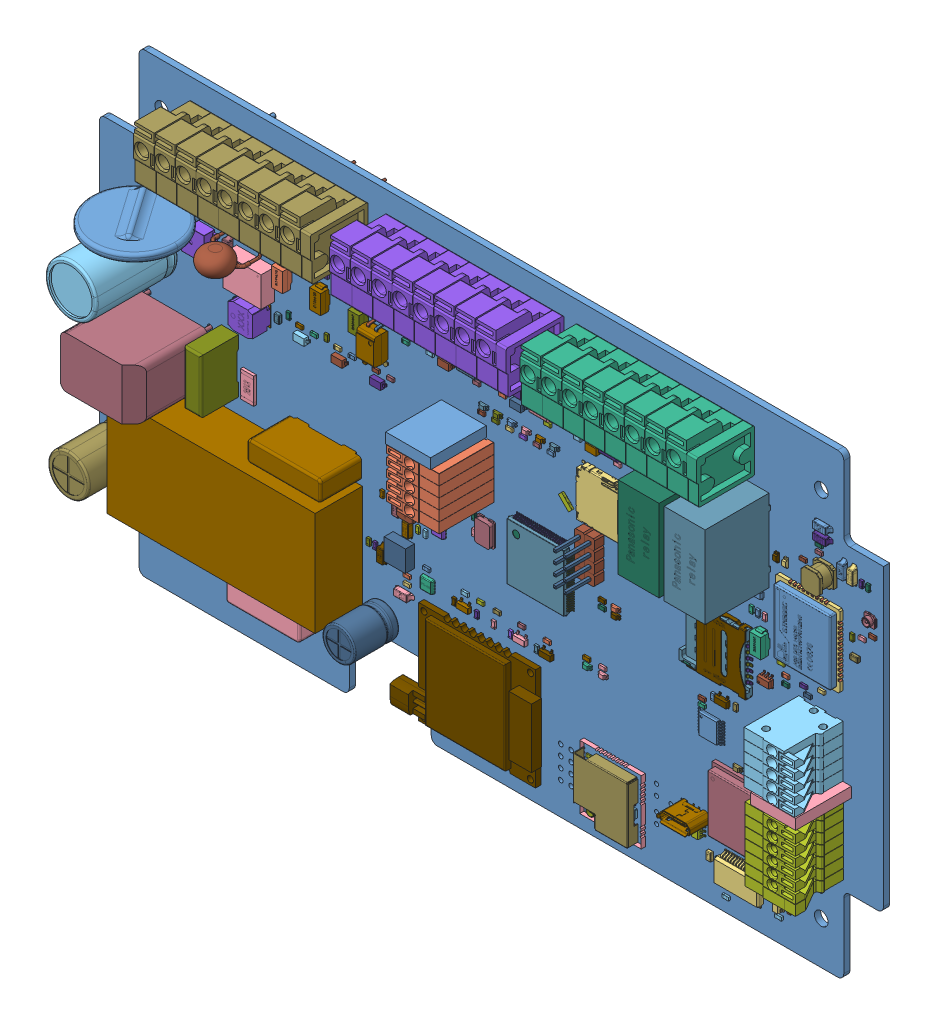
SolidWorks assembly Velvet_Controller_V1.2_2023, configuration Default. Lengths in mm. (continued)
Components (placement in the parent): (continued)
- Velvet_Controller_V1.2_2023(2)^Velvet_Controller_V1.2_2023-1: Velvet_Controller_V1.2_2023(2)^Velvet_Controller_V1.2_2023 [Default] at origin size (191.4 111.4 51.25) (virtual) (continued)
  - R6lr^Velvet_Controller_V1.2_2023(2)_Velvet_Controller_V1.2_2023-1: R6lr^Velvet_Controller_V1.2_2023(2)_Velvet_Controller_V1.2_2023 [Default] at origin size (0.86 1.6 0.51) (virtual)
    - RES 0603^R6lr_Velvet_Controller_V1.2_2023(2)_Velvet_Controller_V1.2_2023-1: RES 0603^R6lr_Velvet_Controller_V1.2_2023(2)_Velvet_Controller_V1.2_2023 [Default] at (107 32.9 0) x (0 1 0) z (1 0 0) size (1.6 0.51 0.86) (virtual)
  - R6io^Velvet_Controller_V1.2_2023(2)_Velvet_Controller_V1.2_2023-1: R6io^Velvet_Controller_V1.2_2023(2)_Velvet_Controller_V1.2_2023 [Default] at origin size (0.86 1.6 0.51) (virtual)
    - RES 0603^R6io_Velvet_Controller_V1.2_2023(2)_Velvet_Controller_V1.2_2023-1: RES 0603^R6io_Velvet_Controller_V1.2_2023(2)_Velvet_Controller_V1.2_2023 [Default] at (46.41 73.1 0) x (0 -1 0) z (-1 0 0) size (1.6 0.51 0.86) (virtual)
  - R6gs^Velvet_Controller_V1.2_2023(2)_Velvet_Controller_V1.2_2023-1: R6gs^Velvet_Controller_V1.2_2023(2)_Velvet_Controller_V1.2_2023 [Default] at origin size (0.86 1.6 0.51) (virtual)
    - RES 0603^R6gs_Velvet_Controller_V1.2_2023(2)_Velvet_Controller_V1.2_2023-1: RES 0603^R6gs_Velvet_Controller_V1.2_2023(2)_Velvet_Controller_V1.2_2023 [Default] at (183.975 73.9 0) x (0 1 0) z (1 0 0) size (1.6 0.51 0.86) (virtual)
  - R5wf^Velvet_Controller_V1.2_2023(2)_Velvet_Controller_V1.2_2023-1: R5wf^Velvet_Controller_V1.2_2023(2)_Velvet_Controller_V1.2_2023 [Default] at origin size (0.86 1.6 0.51) (virtual)
    - RES 0603^R5wf_Velvet_Controller_V1.2_2023(2)_Velvet_Controller_V1.2_2023-1: RES 0603^R5wf_Velvet_Controller_V1.2_2023(2)_Velvet_Controller_V1.2_2023 [Default] at (170.35 12 0) x (0 -1 0) z (-1 0 0) size (1.6 0.51 0.86) (virtual)
  - R5p^Velvet_Controller_V1.2_2023(2)_Velvet_Controller_V1.2_2023-1: R5p^Velvet_Controller_V1.2_2023(2)_Velvet_Controller_V1.2_2023 [Default] at origin size (0.86 1.6 0.51) (virtual)
    - RES 0603^R5p_Velvet_Controller_V1.2_2023(2)_Velvet_Controller_V1.2_2023-1: RES 0603^R5p_Velvet_Controller_V1.2_2023(2)_Velvet_Controller_V1.2_2023 [Default] at (168.4 87.5 -1.5) x (0 1 0) z (-1 0 0) size (1.6 0.51 0.86) (virtual)
  - R5mc^Velvet_Controller_V1.2_2023(2)_Velvet_Controller_V1.2_2023-1: R5mc^Velvet_Controller_V1.2_2023(2)_Velvet_Controller_V1.2_2023 [Default] at origin size (1.6 0.86 0.51) (virtual)
    - RES 0603^R5mc_Velvet_Controller_V1.2_2023(2)_Velvet_Controller_V1.2_2023-1: RES 0603^R5mc_Velvet_Controller_V1.2_2023(2)_Velvet_Controller_V1.2_2023 [Default] at (110.55 76.125 0) x (1 0 0) z (0 -1 0) size (1.6 0.51 0.86) (virtual)
  - R5lr^Velvet_Controller_V1.2_2023(2)_Velvet_Controller_V1.2_2023-1: R5lr^Velvet_Controller_V1.2_2023(2)_Velvet_Controller_V1.2_2023 [Default] at origin size (1.6 0.86 0.51) (virtual)
    - RES 0603^R5lr_Velvet_Controller_V1.2_2023(2)_Velvet_Controller_V1.2_2023-1: RES 0603^R5lr_Velvet_Controller_V1.2_2023(2)_Velvet_Controller_V1.2_2023 [Default] at (109.6 35.8 0) x (1 0 0) z (0 -1 0) size (1.6 0.51 0.86) (virtual)
  - R5io^Velvet_Controller_V1.2_2023(2)_Velvet_Controller_V1.2_2023-1: R5io^Velvet_Controller_V1.2_2023(2)_Velvet_Controller_V1.2_2023 [Default] at origin size (0.86 1.6 0.51) (virtual)
    - RES 0603^R5io_Velvet_Controller_V1.2_2023(2)_Velvet_Controller_V1.2_2023-1: RES 0603^R5io_Velvet_Controller_V1.2_2023(2)_Velvet_Controller_V1.2_2023 [Default] at (79.5 85 0) x (0 1 0) z (1 0 0) size (1.6 0.51 0.86) (virtual)
  - R5gs^Velvet_Controller_V1.2_2023(2)_Velvet_Controller_V1.2_2023-1: R5gs^Velvet_Controller_V1.2_2023(2)_Velvet_Controller_V1.2_2023 [Default] at origin size (1.6 0.86 0.51) (virtual)
    - RES 0603^R5gs_Velvet_Controller_V1.2_2023(2)_Velvet_Controller_V1.2_2023-1: RES 0603^R5gs_Velvet_Controller_V1.2_2023(2)_Velvet_Controller_V1.2_2023 [Default] at (186.5 74.8 0) x (1 0 0) z (0 -1 0) size (1.6 0.51 0.86) (virtual)
  - R4wf^Velvet_Controller_V1.2_2023(2)_Velvet_Controller_V1.2_2023-1: R4wf^Velvet_Controller_V1.2_2023(2)_Velvet_Controller_V1.2_2023 [Default] at origin size (1.6 0.86 0.51) (virtual)
    - RES 0603^R4wf_Velvet_Controller_V1.2_2023(2)_Velvet_Controller_V1.2_2023-1: RES 0603^R4wf_Velvet_Controller_V1.2_2023(2)_Velvet_Controller_V1.2_2023 [Default] at (166.125 5.825 0) x (1 0 0) z (0 -1 0) size (1.6 0.51 0.86) (virtual)
  - R4p^Velvet_Controller_V1.2_2023(2)_Velvet_Controller_V1.2_2023-1: R4p^Velvet_Controller_V1.2_2023(2)_Velvet_Controller_V1.2_2023 [Default] at origin size (1.6 0.86 0.51) (virtual)
    - RES 0603^R4p_Velvet_Controller_V1.2_2023(2)_Velvet_Controller_V1.2_2023-1: RES 0603^R4p_Velvet_Controller_V1.2_2023(2)_Velvet_Controller_V1.2_2023 [Default] at (83.3248 49.0693 -1.5) x (1 0 0) z (0 1 0) size (1.6 0.51 0.86) (virtual)
  - R4mc^Velvet_Controller_V1.2_2023(2)_Velvet_Controller_V1.2_2023-1: R4mc^Velvet_Controller_V1.2_2023(2)_Velvet_Controller_V1.2_2023 [Default] at origin size (0.86 1.6 0.51) (virtual)
    - RES 0603^R4mc_Velvet_Controller_V1.2_2023(2)_Velvet_Controller_V1.2_2023-1: RES 0603^R4mc_Velvet_Controller_V1.2_2023(2)_Velvet_Controller_V1.2_2023 [Default] at (105.65 58.3 -1.5) x (0 1 0) z (-1 0 0) size (1.6 0.51 0.86) (virtual)
  - R4lr^Velvet_Controller_V1.2_2023(2)_Velvet_Controller_V1.2_2023-1: R4lr^Velvet_Controller_V1.2_2023(2)_Velvet_Controller_V1.2_2023 [Default] at origin size (0.86 1.6 0.51) (virtual)
    - RES 0603^R4lr_Velvet_Controller_V1.2_2023(2)_Velvet_Controller_V1.2_2023-1: RES 0603^R4lr_Velvet_Controller_V1.2_2023(2)_Velvet_Controller_V1.2_2023 [Default] at (100.7 32.9 0) x (0 1 0) z (1 0 0) size (1.6 0.51 0.86) (virtual)
  - R4io^Velvet_Controller_V1.2_2023(2)_Velvet_Controller_V1.2_2023-1: R4io^Velvet_Controller_V1.2_2023(2)_Velvet_Controller_V1.2_2023 [Default] at origin size (1.6 0.86 0.51) (virtual)
    - RES 0603^R4io_Velvet_Controller_V1.2_2023(2)_Velvet_Controller_V1.2_2023-1: RES 0603^R4io_Velvet_Controller_V1.2_2023(2)_Velvet_Controller_V1.2_2023 [Default] at (49.11 72.2 0) x (-1 0 0) z (0 1 0) size (1.6 0.51 0.86) (virtual)
  - R4gs^Velvet_Controller_V1.2_2023(2)_Velvet_Controller_V1.2_2023-1: R4gs^Velvet_Controller_V1.2_2023(2)_Velvet_Controller_V1.2_2023 [Default] at origin size (1.6 0.86 0.51) (virtual)
    - RES 0603^R4gs_Velvet_Controller_V1.2_2023(2)_Velvet_Controller_V1.2_2023-1: RES 0603^R4gs_Velvet_Controller_V1.2_2023(2)_Velvet_Controller_V1.2_2023 [Default] at (173.2 56.15 0) x (1 0 0) z (0 -1 0) size (1.6 0.51 0.86) (virtual)
  - R3wf^Velvet_Controller_V1.2_2023(2)_Velvet_Controller_V1.2_2023-1: R3wf^Velvet_Controller_V1.2_2023(2)_Velvet_Controller_V1.2_2023 [Default] at origin size (0.86 1.6 0.51) (virtual)
    - RES 0603^R3wf_Velvet_Controller_V1.2_2023(2)_Velvet_Controller_V1.2_2023-1: RES 0603^R3wf_Velvet_Controller_V1.2_2023(2)_Velvet_Controller_V1.2_2023 [Default] at (168.725 8.575 0) x (0 -1 0) z (-1 0 0) size (1.6 0.51 0.86) (virtual)
  - R3p^Velvet_Controller_V1.2_2023(2)_Velvet_Controller_V1.2_2023-1: R3p^Velvet_Controller_V1.2_2023(2)_Velvet_Controller_V1.2_2023 [Default] at origin size (1.6 0.86 0.51) (virtual)
    - RES 0603^R3p_Velvet_Controller_V1.2_2023(2)_Velvet_Controller_V1.2_2023-1: RES 0603^R3p_Velvet_Controller_V1.2_2023(2)_Velvet_Controller_V1.2_2023 [Default] at (172.1 84.4 -1.5) x (1 0 0) z (0 1 0) size (1.6 0.51 0.86) (virtual)
  - R3lr^Velvet_Controller_V1.2_2023(2)_Velvet_Controller_V1.2_2023-1: R3lr^Velvet_Controller_V1.2_2023(2)_Velvet_Controller_V1.2_2023 [Default] at origin size (1.6 0.86 0.51) (virtual)
    - RES 0603^R3lr_Velvet_Controller_V1.2_2023(2)_Velvet_Controller_V1.2_2023-1: RES 0603^R3lr_Velvet_Controller_V1.2_2023(2)_Velvet_Controller_V1.2_2023 [Default] at (103.3 35.9 0) x (1 0 0) z (0 -1 0) size (1.6 0.51 0.86) (virtual)
  - R3io^Velvet_Controller_V1.2_2023(2)_Velvet_Controller_V1.2_2023-1: R3io^Velvet_Controller_V1.2_2023(2)_Velvet_Controller_V1.2_2023 [Default] at origin size (0.86 1.6 0.51) (virtual)
    - RES 0603^R3io_Velvet_Controller_V1.2_2023(2)_Velvet_Controller_V1.2_2023-1: RES 0603^R3io_Velvet_Controller_V1.2_2023(2)_Velvet_Controller_V1.2_2023 [Default] at (46.41 86.4 0) x (0 -1 0) z (-1 0 0) size (1.6 0.51 0.86) (virtual)
  - R3gs^Velvet_Controller_V1.2_2023(2)_Velvet_Controller_V1.2_2023-1: R3gs^Velvet_Controller_V1.2_2023(2)_Velvet_Controller_V1.2_2023 [Default] at origin size (1.6 0.86 0.51) (virtual)
    - RES 0603^R3gs_Velvet_Controller_V1.2_2023(2)_Velvet_Controller_V1.2_2023-1: RES 0603^R3gs_Velvet_Controller_V1.2_2023(2)_Velvet_Controller_V1.2_2023 [Default] at (167.775 55.775 0) x (1 0 0) z (0 -1 0) size (1.6 0.51 0.86) (virtual)
  - R2wf^Velvet_Controller_V1.2_2023(2)_Velvet_Controller_V1.2_2023-1: R2wf^Velvet_Controller_V1.2_2023(2)_Velvet_Controller_V1.2_2023 [Default] at origin size (1.6 0.86 0.51) (virtual)
    - RES 0603^R2wf_Velvet_Controller_V1.2_2023(2)_Velvet_Controller_V1.2_2023-1: RES 0603^R2wf_Velvet_Controller_V1.2_2023(2)_Velvet_Controller_V1.2_2023 [Default] at (159.55 32.25 0) x (-1 0 0) z (0 1 0) size (1.6 0.51 0.86) (virtual)
  - R2p^Velvet_Controller_V1.2_2023(2)_Velvet_Controller_V1.2_2023-1: R2p^Velvet_Controller_V1.2_2023(2)_Velvet_Controller_V1.2_2023 [Default] at origin size (0.86 1.6 0.51) (virtual)
    - RES 0603^R2p_Velvet_Controller_V1.2_2023(2)_Velvet_Controller_V1.2_2023-1: RES 0603^R2p_Velvet_Controller_V1.2_2023(2)_Velvet_Controller_V1.2_2023 [Default] at (14.5 82 0) x (0 -1 0) z (-1 0 0) size (1.6 0.51 0.86) (virtual)
  - R2lr^Velvet_Controller_V1.2_2023(2)_Velvet_Controller_V1.2_2023-1: R2lr^Velvet_Controller_V1.2_2023(2)_Velvet_Controller_V1.2_2023 [Default] at origin size (0.86 1.6 0.51) (virtual)
    - RES 0603^R2lr_Velvet_Controller_V1.2_2023(2)_Velvet_Controller_V1.2_2023-1: RES 0603^R2lr_Velvet_Controller_V1.2_2023(2)_Velvet_Controller_V1.2_2023 [Default] at (86.9 32.9 0) x (0 1 0) z (1 0 0) size (1.6 0.51 0.86) (virtual)
  - R2io^Velvet_Controller_V1.2_2023(2)_Velvet_Controller_V1.2_2023-1: R2io^Velvet_Controller_V1.2_2023(2)_Velvet_Controller_V1.2_2023 [Default] at origin size (0.8 1.6 0.5) (virtual)
    - CAP 0603 (1608)^R2io_Velvet_Controller_V1.2_2023(2)_Velvet_Controller_V1.2_2023-1: CAP 0603 (1608)^R2io_Velvet_Controller_V1.2_2023(2)_Velvet_Controller_V1.2_2023 [Default] at (44.5 85.6 0) x (0 1 0) z (1 0 0) size (1.6 0.5 0.8) (virtual)
  - R2gs^Velvet_Controller_V1.2_2023(2)_Velvet_Controller_V1.2_2023-1: R2gs^Velvet_Controller_V1.2_2023(2)_Velvet_Controller_V1.2_2023 [Default] at origin size (1.6 0.86 0.51) (virtual)
    - RES 0603^R2gs_Velvet_Controller_V1.2_2023(2)_Velvet_Controller_V1.2_2023-1: RES 0603^R2gs_Velvet_Controller_V1.2_2023(2)_Velvet_Controller_V1.2_2023 [Default] at (167.775 57.6 0) x (1 0 0) z (0 -1 0) size (1.6 0.51 0.86) (virtual)
  - R1wf^Velvet_Controller_V1.2_2023(2)_Velvet_Controller_V1.2_2023-1: R1wf^Velvet_Controller_V1.2_2023(2)_Velvet_Controller_V1.2_2023 [Default] at origin size (0.86 1.6 0.51) (virtual)
    - RES 0603^R1wf_Velvet_Controller_V1.2_2023(2)_Velvet_Controller_V1.2_2023-1: RES 0603^R1wf_Velvet_Controller_V1.2_2023(2)_Velvet_Controller_V1.2_2023 [Default] at (168.75 11.975 0) x (0 1 0) z (1 0 0) size (1.6 0.51 0.86) (virtual)
  - R1p^Velvet_Controller_V1.2_2023(2)_Velvet_Controller_V1.2_2023-1: R1p^Velvet_Controller_V1.2_2023(2)_Velvet_Controller_V1.2_2023 [Default] at origin size (3.2 6.4 0.65) (virtual)
    - Resistor SMD 2512^R1p_Velvet_Controller_V1.2_2023(2)_Velvet_Controller_V1.2_2023-1: Resistor SMD 2512^R1p_Velvet_Controller_V1.2_2023(2)_Velvet_Controller_V1.2_2023 [Default] at (36.7 53.2 0) x (0 1 0) z (0 0 1) size (6.4 3.2 0.65) (virtual)
  - R1lr^Velvet_Controller_V1.2_2023(2)_Velvet_Controller_V1.2_2023-1: R1lr^Velvet_Controller_V1.2_2023(2)_Velvet_Controller_V1.2_2023 [Default] at origin size (1.6 0.86 0.51) (virtual)
    - RES 0603^R1lr_Velvet_Controller_V1.2_2023(2)_Velvet_Controller_V1.2_2023-1: RES 0603^R1lr_Velvet_Controller_V1.2_2023(2)_Velvet_Controller_V1.2_2023 [Default] at (89.5 35.9 0) x (1 0 0) z (0 -1 0) size (1.6 0.51 0.86) (virtual)
  - R1io^Velvet_Controller_V1.2_2023(2)_Velvet_Controller_V1.2_2023-1: R1io^Velvet_Controller_V1.2_2023(2)_Velvet_Controller_V1.2_2023 [Default] at origin size (1.6 0.86 0.51) (virtual)
    - RES 0603^R1io_Velvet_Controller_V1.2_2023(2)_Velvet_Controller_V1.2_2023-1: RES 0603^R1io_Velvet_Controller_V1.2_2023(2)_Velvet_Controller_V1.2_2023 [Default] at (75 81.825 0) x (-1 0 0) z (0 1 0) size (1.6 0.51 0.86) (virtual)
  - R1gs^Velvet_Controller_V1.2_2023(2)_Velvet_Controller_V1.2_2023-1: R1gs^Velvet_Controller_V1.2_2023(2)_Velvet_Controller_V1.2_2023 [Default] at origin size (1.6 0.86 0.51) (virtual)
    - RES 0603^R1gs_Velvet_Controller_V1.2_2023(2)_Velvet_Controller_V1.2_2023-1: RES 0603^R1gs_Velvet_Controller_V1.2_2023(2)_Velvet_Controller_V1.2_2023 [Default] at (166.725 59.8 0) x (-1 0 0) z (0 1 0) size (1.6 0.51 0.86) (virtual)
  - L5p^Velvet_Controller_V1.2_2023(2)_Velvet_Controller_V1.2_2023-1: L5p^Velvet_Controller_V1.2_2023(2)_Velvet_Controller_V1.2_2023 [Default] at origin size (6 6 4.5) (virtual)
    - vls6045ex^L5p_Velvet_Controller_V1.2_2023(2)_Velvet_Controller_V1.2_2023-1: vls6045ex^L5p_Velvet_Controller_V1.2_2023(2)_Velvet_Controller_V1.2_2023 [Default] at (38.9 70.5 2.25) x (1 0 0) z (0 -1 0) size (6 4.5 6) (virtual)
      - VLS6045EX_C(3Dmodel)^vls6045ex_L5p_Velvet_Controller_V1.2_2023(2)_Velvet_Controller_V1.2_2023-1: VLS6045EX_C(3Dmodel)^vls6045ex_L5p_Velvet_Controller_V1.2_2023(2)_Velvet_Controller_V1.2_2023 [Default] at origin size (6 4.48 6) (virtual)
      - VLS6045EX_T(3Dmodel)^vls6045ex_L5p_Velvet_Controller_V1.2_2023(2)_Velvet_Controller_V1.2_2023-1: VLS6045EX_T(3Dmodel)^vls6045ex_L5p_Velvet_Controller_V1.2_2023(2)_Velvet_Controller_V1.2_2023 [Default] at (0 -2.185 0) size (6 0.15 4.8) (virtual)
  - L4p^Velvet_Controller_V1.2_2023(2)_Velvet_Controller_V1.2_2023-1: L4p^Velvet_Controller_V1.2_2023(2)_Velvet_Controller_V1.2_2023 [Default] at origin size (5.2 5.2 2.2) (virtual)
    - 6303148784^L4p_Velvet_Controller_V1.2_2023(2)_Velvet_Controller_V1.2_2023-1: 6303148784^L4p_Velvet_Controller_V1.2_2023(2)_Velvet_Controller_V1.2_2023 [Default] at (74.3 37.35 0) size (5.2 5.2 2.2) (virtual)
      - Extruded-2^6303148784_L4p_Velvet_Controller_V1.2_2023(2)_Velvet_Controller_V1.2_2023-1: Extruded-2^6303148784_L4p_Velvet_Controller_V1.2_2023(2)_Velvet_Controller_V1.2_2023 [Default] at origin size (5.2 5.2 2.2) (virtual)
  - L3p^Velvet_Controller_V1.2_2023(2)_Velvet_Controller_V1.2_2023-1: L3p^Velvet_Controller_V1.2_2023(2)_Velvet_Controller_V1.2_2023 [Default] at origin size (4 4 3) (virtual)
    - ASPI-4030S^L3p_Velvet_Controller_V1.2_2023(2)_Velvet_Controller_V1.2_2023-1: ASPI-4030S^L3p_Velvet_Controller_V1.2_2023(2)_Velvet_Controller_V1.2_2023 [Default] at (77.4497 48.5943 0) x (0 -1 0) z (-1 0 0) size (4 3 4) (virtual)
  - L2p^Velvet_Controller_V1.2_2023(2)_Velvet_Controller_V1.2_2023-1: L2p^Velvet_Controller_V1.2_2023(2)_Velvet_Controller_V1.2_2023 [Default] at origin size (5 5 4) (virtual)
    - SRN5040^L2p_Velvet_Controller_V1.2_2023(2)_Velvet_Controller_V1.2_2023-1: SRN5040^L2p_Velvet_Controller_V1.2_2023(2)_Velvet_Controller_V1.2_2023 [Default] at (177.5 84.2 0) x (1 0 0) z (0 -1 0) size (5 4 5) (virtual)
  - L1p^Velvet_Controller_V1.2_2023(2)_Velvet_Controller_V1.2_2023-1: L1p^Velvet_Controller_V1.2_2023(2)_Velvet_Controller_V1.2_2023 [Default] at origin size (18 12.5 24) (virtual)
    - RN212-x-02^L1p_Velvet_Controller_V1.2_2023(2)_Velvet_Controller_V1.2_2023-1: RN212-x-02^L1p_Velvet_Controller_V1.2_2023(2)_Velvet_Controller_V1.2_2023 [Default] at (19.5 55.775 20) x (-1 0 0) z (0 0 -1) size (18 12.5 24) (virtual)
  - K2io^Velvet_Controller_V1.2_2023(2)_Velvet_Controller_V1.2_2023-1: K2io^Velvet_Controller_V1.2_2023(2)_Velvet_Controller_V1.2_2023 [Default] at origin size (10 20 19.8) (virtual)
    - ALQ1 (STEP)^K2io_Velvet_Controller_V1.2_2023(2)_Velvet_Controller_V1.2_2023-1: ALQ1 (STEP)^K2io_Velvet_Controller_V1.2_2023(2)_Velvet_Controller_V1.2_2023 [Default] at (158.85 84.35 0) x (0 1 0) z (0 0 1) size (20 10 19.8) (virtual)
  - K1io^Velvet_Controller_V1.2_2023(2)_Velvet_Controller_V1.2_2023-1: K1io^Velvet_Controller_V1.2_2023(2)_Velvet_Controller_V1.2_2023 [Default] at origin size (10 20 19.8) (virtual)
    - ALQ1 (STEP)^K1io_Velvet_Controller_V1.2_2023(2)_Velvet_Controller_V1.2_2023-1: ALQ1 (STEP)^K1io_Velvet_Controller_V1.2_2023(2)_Velvet_Controller_V1.2_2023 [Default] at (147.61 84.35 0) x (0 1 0) z (0 0 1) size (20 10 19.8) (virtual)
  - FU1p^Velvet_Controller_V1.2_2023(2)_Velvet_Controller_V1.2_2023-1: FU1p^Velvet_Controller_V1.2_2023(2)_Velvet_Controller_V1.2_2023 [Default] at origin size (12.11 2.61 6.6) (virtual)
    - 0ZRP0500FF1A^FU1p_Velvet_Controller_V1.2_2023(2)_Velvet_Controller_V1.2_2023-1: 0ZRP0500FF1A^FU1p_Velvet_Controller_V1.2_2023(2)_Velvet_Controller_V1.2_2023 [Default] at (17.9 92.6 0) x (1 0 0) z (0 0 1) size (12.1 2.6 6.6) (virtual)
      - Body^0ZRP0500FF1A_FU1p_Velvet_Controller_V1.2_2023(2)_Velvet_Controller_V1.2_2023-1: Body^0ZRP0500FF1A_FU1p_Velvet_Controller_V1.2_2023(2)_Velvet_Controller_V1.2_2023 [Default] at (0 0 0.1) size (3 0.8 3) (virtual)
      - Leads^0ZRP0500FF1A_FU1p_Velvet_Controller_V1.2_2023(2)_Velvet_Controller_V1.2_2023-1: Leads^0ZRP0500FF1A_FU1p_Velvet_Controller_V1.2_2023(2)_Velvet_Controller_V1.2_2023 [Default] at origin size (11.01 2.21 5.1) (virtual)
  - DD4mc^Velvet_Controller_V1.2_2023(2)_Velvet_Controller_V1.2_2023-1: DD4mc^Velvet_Controller_V1.2_2023(2)_Velvet_Controller_V1.2_2023 [Default] at origin size (3 2.5 1.1) (virtual)
    - SOT-23-5^DD4mc_Velvet_Controller_V1.2_2023(2)_Velvet_Controller_V1.2_2023-1: SOT-23-5^DD4mc_Velvet_Controller_V1.2_2023(2)_Velvet_Controller_V1.2_2023 [Default] at (152.55 44.75 0.55) x (1 0 0) z (0 -1 0) size (3 1.1 2.5) (virtual)
  - DD3mc^Velvet_Controller_V1.2_2023(2)_Velvet_Controller_V1.2_2023-1: DD3mc^Velvet_Controller_V1.2_2023(2)_Velvet_Controller_V1.2_2023 [Default] at origin size (6.4 5 1.1) (virtual)
    - TSSOP-16-1^DD3mc_Velvet_Controller_V1.2_2023(2)_Velvet_Controller_V1.2_2023-1: TSSOP-16-1^DD3mc_Velvet_Controller_V1.2_2023(2)_Velvet_Controller_V1.2_2023 [Default] at (149.55 37.75 0) size (6.4 5 1.1) (virtual)
  - DD3lr^Velvet_Controller_V1.2_2023(2)_Velvet_Controller_V1.2_2023-1: DD3lr^Velvet_Controller_V1.2_2023(2)_Velvet_Controller_V1.2_2023 [Default] at origin size (1.6 1.63 0.58) (virtual)
    - SOT-563^DD3lr_Velvet_Controller_V1.2_2023(2)_Velvet_Controller_V1.2_2023-1: SOT-563^DD3lr_Velvet_Controller_V1.2_2023(2)_Velvet_Controller_V1.2_2023 [Default] at (93.5043 16.975 -1.5) x (1 0 0) z (0 1 0) size (1.6 0.58 1.63) (virtual)
  - DD2wf^Velvet_Controller_V1.2_2023(2)_Velvet_Controller_V1.2_2023-1: DD2wf^Velvet_Controller_V1.2_2023(2)_Velvet_Controller_V1.2_2023 [Default] at origin size (10.41 8.12 2.03) (virtual)
    - PG-SSOP-28-800^DD2wf_Velvet_Controller_V1.2_2023(2)_Velvet_Controller_V1.2_2023-1: PG-SSOP-28-800^DD2wf_Velvet_Controller_V1.2_2023(2)_Velvet_Controller_V1.2_2023 [Default] at (157.225 9.4 0) x (0 -1 0) z (0 0 1) size (8.12 10.41 2.03) (virtual)
  - DD2lr^Velvet_Controller_V1.2_2023(2)_Velvet_Controller_V1.2_2023-1: DD2lr^Velvet_Controller_V1.2_2023(2)_Velvet_Controller_V1.2_2023 [Default] at origin size (15 15.75 3.52) (virtual)
    - 3D_RAK3172^DD2lr_Velvet_Controller_V1.2_2023(2)_Velvet_Controller_V1.2_2023-1: 3D_RAK3172^DD2lr_Velvet_Controller_V1.2_2023(2)_Velvet_Controller_V1.2_2023 [Default] at (133.2551 19.6 1) x (-1 0 0) z (0 0 1) size (15 15.75 3.52) (virtual)
      - Board-1^3D_RAK3172_DD2lr_Velvet_Controller_V1.2_2023(2)_Velvet_Controller_V1.2_2023-1: Board-1^3D_RAK3172_DD2lr_Velvet_Controller_V1.2_2023(2)_Velvet_Controller_V1.2_2023 [Default] at origin size (15 15.75 1.01) (virtual)
        - Open CASCADE STEP translator 6.8 1.1.1^Board-1_3D_RAK3172_DD2lr_Velvet_Controller_V1.2_2023(2)_Velvet_Controller_V1.2_2023-1: Open CASCADE STEP translator 6.8 1.1.1^Board-1_3D_RAK3172_DD2lr_Velvet_Controller_V1.2_2023(2)_Velvet_Controller_V1.2_2023 [Default] at (0 0 -1.014) size (15 15.75 1.01) (virtual)
          - Open CASCADE STEP translator 6.8 1.1.1.1^Open CASCADE STEP translator 6.8 1.1.1_Board-1_3D_RAK3172_DD2lr_Velvet_Controller_V1.2_2023(2)_Velvet_Controller_V1.2_2023-1: Open CASCADE STEP translator 6.8 1.1.1.1^Open CASCADE STEP translator 6.8 1.1.1_Board-1_3D_RAK3172_DD2lr_Velvet_Controller_V1.2_2023(2)_Velvet_Controller_V1.2_2023 [Default] at origin size (15 15.75 1.01) (virtual)
      - R11^3D_RAK3172_DD2lr_Velvet_Controller_V1.2_2023(2)_Velvet_Controller_V1.2_2023-1: R11^3D_RAK3172_DD2lr_Velvet_Controller_V1.2_2023(2)_Velvet_Controller_V1.2_2023 [Default] at origin size (0.6 0.3 0.3) (virtual)
        - 0201_SMD_Capacitor^R11_3D_RAK3172_DD2lr_Velvet_Controller_V1.2_2023(2)_Velvet_Controller_V1.2_2023-1: 0201_SMD_Capacitor^R11_3D_RAK3172_DD2lr_Velvet_Controller_V1.2_2023(2)_Velvet_Controller_V1.2_2023 [Default] at (3.4751 6.9342 0.2794) x (-1 0 0) z (0 0 1) size (0.6 0.3 0.3) (virtual)
      - U2^3D_RAK3172_DD2lr_Velvet_Controller_V1.2_2023(2)_Velvet_Controller_V1.2_2023-1: U2^3D_RAK3172_DD2lr_Velvet_Controller_V1.2_2023(2)_Velvet_Controller_V1.2_2023 [Default] at origin size (0.99 1.02 0.75) (virtual)
        - 6590464912^U2_3D_RAK3172_DD2lr_Velvet_Controller_V1.2_2023(2)_Velvet_Controller_V1.2_2023-1: 6590464912^U2_3D_RAK3172_DD2lr_Velvet_Controller_V1.2_2023(2)_Velvet_Controller_V1.2_2023 [Default] at (5.4483 13.05 0) size (0.99 1.02 0.75) (virtual)
          - Extruded-3^6590464912_U2_3D_RAK3172_DD2lr_Velvet_Controller_V1.2_2023(2)_Velvet_Controller_V1.2_2023-1: Extruded-3^6590464912_U2_3D_RAK3172_DD2lr_Velvet_Controller_V1.2_2023(2)_Velvet_Controller_V1.2_2023 [Default] at origin size (0.99 1.02 0.75) (virtual)
      - R4^3D_RAK3172_DD2lr_Velvet_Controller_V1.2_2023(2)_Velvet_Controller_V1.2_2023-1: R4^3D_RAK3172_DD2lr_Velvet_Controller_V1.2_2023(2)_Velvet_Controller_V1.2_2023 [Default] at origin size (0.68 0.33 0.34) (virtual)
        - R0201^R4_3D_RAK3172_DD2lr_Velvet_Controller_V1.2_2023(2)_Velvet_Controller_V1.2_2023-1: R0201^R4_3D_RAK3172_DD2lr_Velvet_Controller_V1.2_2023(2)_Velvet_Controller_V1.2_2023 [Default] at (3.9176 5.9192 0) x (1 0 0) z (0 -1 0) size (0.68 0.34 0.33) (virtual)
      - R3^3D_RAK3172_DD2lr_Velvet_Controller_V1.2_2023(2)_Velvet_Controller_V1.2_2023-1: R3^3D_RAK3172_DD2lr_Velvet_Controller_V1.2_2023(2)_Velvet_Controller_V1.2_2023 [Default] at origin size (0.33 0.68 0.34) (virtual)
        - R0201^R3_3D_RAK3172_DD2lr_Velvet_Controller_V1.2_2023(2)_Velvet_Controller_V1.2_2023-1: R0201^R3_3D_RAK3172_DD2lr_Velvet_Controller_V1.2_2023(2)_Velvet_Controller_V1.2_2023 [Default] at (4.1676 5.6692 0) x (0 1 0) z (1 0 0) size (0.68 0.34 0.33) (virtual)
      - L2^3D_RAK3172_DD2lr_Velvet_Controller_V1.2_2023(2)_Velvet_Controller_V1.2_2023-1: L2^3D_RAK3172_DD2lr_Velvet_Controller_V1.2_2023(2)_Velvet_Controller_V1.2_2023 [Default] at origin size (1.15 0.55 0.41) (virtual)
        - RES_1005-0402^L2_3D_RAK3172_DD2lr_Velvet_Controller_V1.2_2023(2)_Velvet_Controller_V1.2_2023-1: RES_1005-0402^L2_3D_RAK3172_DD2lr_Velvet_Controller_V1.2_2023(2)_Velvet_Controller_V1.2_2023 [Default] at (2.2661 6.0198 0) x (1 0 0) z (0 -1 0) size (1.15 0.41 0.55) (virtual)
      - C10^3D_RAK3172_DD2lr_Velvet_Controller_V1.2_2023(2)_Velvet_Controller_V1.2_2023-1: C10^3D_RAK3172_DD2lr_Velvet_Controller_V1.2_2023(2)_Velvet_Controller_V1.2_2023 [Default] at origin size (0.6 0.3 0.3) (virtual)
        - 0201_SMD_Capacitor^C10_3D_RAK3172_DD2lr_Velvet_Controller_V1.2_2023(2)_Velvet_Controller_V1.2_2023-1: 0201_SMD_Capacitor^C10_3D_RAK3172_DD2lr_Velvet_Controller_V1.2_2023(2)_Velvet_Controller_V1.2_2023 [Default] at (7.1835 13.462 0.2794) x (-1 0 0) z (0 0 1) size (0.6 0.3 0.3) (virtual)
      - C9^3D_RAK3172_DD2lr_Velvet_Controller_V1.2_2023(2)_Velvet_Controller_V1.2_2023-1: C9^3D_RAK3172_DD2lr_Velvet_Controller_V1.2_2023(2)_Velvet_Controller_V1.2_2023 [Default] at origin size (0.6 0.3 0.3) (virtual)
        - 0201_SMD_Capacitor^C9_3D_RAK3172_DD2lr_Velvet_Controller_V1.2_2023(2)_Velvet_Controller_V1.2_2023-1: 0201_SMD_Capacitor^C9_3D_RAK3172_DD2lr_Velvet_Controller_V1.2_2023(2)_Velvet_Controller_V1.2_2023 [Default] at (7.1835 13.97 0.2794) x (-1 0 0) z (0 0 1) size (0.6 0.3 0.3) (virtual)
      - C8^3D_RAK3172_DD2lr_Velvet_Controller_V1.2_2023(2)_Velvet_Controller_V1.2_2023-1: C8^3D_RAK3172_DD2lr_Velvet_Controller_V1.2_2023(2)_Velvet_Controller_V1.2_2023 [Default] at origin size (0.6 0.3 0.3) (virtual)
        - 0201_SMD_Capacitor^C8_3D_RAK3172_DD2lr_Velvet_Controller_V1.2_2023(2)_Velvet_Controller_V1.2_2023-1: 0201_SMD_Capacitor^C8_3D_RAK3172_DD2lr_Velvet_Controller_V1.2_2023(2)_Velvet_Controller_V1.2_2023 [Default] at (7.1835 12.954 0.2794) x (-1 0 0) z (0 0 1) size (0.6 0.3 0.3) (virtual)
      - C7^3D_RAK3172_DD2lr_Velvet_Controller_V1.2_2023(2)_Velvet_Controller_V1.2_2023-1: C7^3D_RAK3172_DD2lr_Velvet_Controller_V1.2_2023(2)_Velvet_Controller_V1.2_2023 [Default] at origin size (0.6 0.3 0.3) (virtual)
        - 0201_SMD_Capacitor^C7_3D_RAK3172_DD2lr_Velvet_Controller_V1.2_2023(2)_Velvet_Controller_V1.2_2023-1: 0201_SMD_Capacitor^C7_3D_RAK3172_DD2lr_Velvet_Controller_V1.2_2023(2)_Velvet_Controller_V1.2_2023 [Default] at (6.0793 11.938 0.2794) x (1 0 0) z (0 0 1) size (0.6 0.3 0.3) (virtual)
      - C6^3D_RAK3172_DD2lr_Velvet_Controller_V1.2_2023(2)_Velvet_Controller_V1.2_2023-1: C6^3D_RAK3172_DD2lr_Velvet_Controller_V1.2_2023(2)_Velvet_Controller_V1.2_2023 [Default] at origin size (0.6 0.3 0.3) (virtual)
        - 0201_SMD_Capacitor^C6_3D_RAK3172_DD2lr_Velvet_Controller_V1.2_2023(2)_Velvet_Controller_V1.2_2023-1: 0201_SMD_Capacitor^C6_3D_RAK3172_DD2lr_Velvet_Controller_V1.2_2023(2)_Velvet_Controller_V1.2_2023 [Default] at (3.8855 13.5541 0.2794) x (-1 0 0) z (0 0 1) size (0.6 0.3 0.3) (virtual)
      - CON1^3D_RAK3172_DD2lr_Velvet_Controller_V1.2_2023(2)_Velvet_Controller_V1.2_2023-1: CON1^3D_RAK3172_DD2lr_Velvet_Controller_V1.2_2023(2)_Velvet_Controller_V1.2_2023 [Default] at origin size (3.4 3.1 1.25) (virtual)
        - UFL-R-SMD^CON1_3D_RAK3172_DD2lr_Velvet_Controller_V1.2_2023(2)_Velvet_Controller_V1.2_2023-1: UFL-R-SMD^CON1_3D_RAK3172_DD2lr_Velvet_Controller_V1.2_2023(2)_Velvet_Controller_V1.2_2023 [Default] at (11.3537 12.7757 0) x (1 0 0) z (0 0 1) size (3.4 3.1 1.25) (virtual)
          - Part_525^UFL-R-SMD_CON1_3D_RAK3172_DD2lr_Velvet_Controller_V1.2_2023(2)_Velvet_Controller_V1.2_2023-1: Part_525^UFL-R-SMD_CON1_3D_RAK3172_DD2lr_Velvet_Controller_V1.2_2023(2)_Velvet_Controller_V1.2_2023 [Default] at origin size (3 2.6 0.35) (virtual)
          - Part_739^UFL-R-SMD_CON1_3D_RAK3172_DD2lr_Velvet_Controller_V1.2_2023(2)_Velvet_Controller_V1.2_2023-1: Part_739^UFL-R-SMD_CON1_3D_RAK3172_DD2lr_Velvet_Controller_V1.2_2023(2)_Velvet_Controller_V1.2_2023 [Default] at origin size (2 2 0.9) (virtual)
          - Part_578^UFL-R-SMD_CON1_3D_RAK3172_DD2lr_Velvet_Controller_V1.2_2023(2)_Velvet_Controller_V1.2_2023-1: Part_578^UFL-R-SMD_CON1_3D_RAK3172_DD2lr_Velvet_Controller_V1.2_2023(2)_Velvet_Controller_V1.2_2023 [Default] at origin size (0.6 0.5 0.1) (virtual)
          - Part_540^UFL-R-SMD_CON1_3D_RAK3172_DD2lr_Velvet_Controller_V1.2_2023(2)_Velvet_Controller_V1.2_2023-1: Part_540^UFL-R-SMD_CON1_3D_RAK3172_DD2lr_Velvet_Controller_V1.2_2023(2)_Velvet_Controller_V1.2_2023 [Default] at origin size (0.4 1.8 0.1) (virtual)
          - Part_562^UFL-R-SMD_CON1_3D_RAK3172_DD2lr_Velvet_Controller_V1.2_2023(2)_Velvet_Controller_V1.2_2023-1: Part_562^UFL-R-SMD_CON1_3D_RAK3172_DD2lr_Velvet_Controller_V1.2_2023(2)_Velvet_Controller_V1.2_2023 [Default] at origin size (0.4 1.8 0.1) (virtual)
          - Part_555^UFL-R-SMD_CON1_3D_RAK3172_DD2lr_Velvet_Controller_V1.2_2023(2)_Velvet_Controller_V1.2_2023-1: Part_555^UFL-R-SMD_CON1_3D_RAK3172_DD2lr_Velvet_Controller_V1.2_2023(2)_Velvet_Controller_V1.2_2023 [Default] at origin size (0.6 0.5 0.1) (virtual)
      - C4^3D_RAK3172_DD2lr_Velvet_Controller_V1.2_2023(2)_Velvet_Controller_V1.2_2023-1: C4^3D_RAK3172_DD2lr_Velvet_Controller_V1.2_2023(2)_Velvet_Controller_V1.2_2023 [Default] at origin size (0.6 0.3 0.3) (virtual)
        - 0201_SMD_Capacitor^C4_3D_RAK3172_DD2lr_Velvet_Controller_V1.2_2023(2)_Velvet_Controller_V1.2_2023-1: 0201_SMD_Capacitor^C4_3D_RAK3172_DD2lr_Velvet_Controller_V1.2_2023(2)_Velvet_Controller_V1.2_2023 [Default] at (3.7799 9.398 0.2794) x (-1 0 0) z (0 0 1) size (0.6 0.3 0.3) (virtual)
      - U1^3D_RAK3172_DD2lr_Velvet_Controller_V1.2_2023(2)_Velvet_Controller_V1.2_2023-1: U1^3D_RAK3172_DD2lr_Velvet_Controller_V1.2_2023(2)_Velvet_Controller_V1.2_2023 [Default] at origin size (7.02 7.02 0.8) (virtual)
        - QFN48_7x7^U1_3D_RAK3172_DD2lr_Velvet_Controller_V1.2_2023(2)_Velvet_Controller_V1.2_2023-1: QFN48_7x7^U1_3D_RAK3172_DD2lr_Velvet_Controller_V1.2_2023(2)_Velvet_Controller_V1.2_2023 [Default] at (8.8366 6.9818 0) x (0 1 0) z (1 0 0) size (7.02 0.8 7.02) (virtual)
      - X1^3D_RAK3172_DD2lr_Velvet_Controller_V1.2_2023(2)_Velvet_Controller_V1.2_2023-1: X1^3D_RAK3172_DD2lr_Velvet_Controller_V1.2_2023(2)_Velvet_Controller_V1.2_2023 [Default] at origin size (1.61 2.01 0.71) (virtual)
        - NT2016SA^X1_3D_RAK3172_DD2lr_Velvet_Controller_V1.2_2023(2)_Velvet_Controller_V1.2_2023-1: NT2016SA^X1_3D_RAK3172_DD2lr_Velvet_Controller_V1.2_2023(2)_Velvet_Controller_V1.2_2023 [Default] at (1.7496 8.4946 0) x (0 1 0) z (1 0 0) size (2.01 0.71 1.61) (virtual)
      - C43^3D_RAK3172_DD2lr_Velvet_Controller_V1.2_2023(2)_Velvet_Controller_V1.2_2023-1: C43^3D_RAK3172_DD2lr_Velvet_Controller_V1.2_2023(2)_Velvet_Controller_V1.2_2023 [Default] at origin size (0.6 0.3 0.3) (virtual)
        - 0201_SMD_Capacitor^C43_3D_RAK3172_DD2lr_Velvet_Controller_V1.2_2023(2)_Velvet_Controller_V1.2_2023-1: 0201_SMD_Capacitor^C43_3D_RAK3172_DD2lr_Velvet_Controller_V1.2_2023(2)_Velvet_Controller_V1.2_2023 [Default] at (3.7799 9.9822 0.2794) x (-1 0 0) z (0 0 1) size (0.6 0.3 0.3) (virtual)
      - C42^3D_RAK3172_DD2lr_Velvet_Controller_V1.2_2023(2)_Velvet_Controller_V1.2_2023-1: C42^3D_RAK3172_DD2lr_Velvet_Controller_V1.2_2023(2)_Velvet_Controller_V1.2_2023 [Default] at origin size (0.3 0.6 0.3) (virtual)
        - 0201_SMD_Capacitor^C42_3D_RAK3172_DD2lr_Velvet_Controller_V1.2_2023(2)_Velvet_Controller_V1.2_2023-1: 0201_SMD_Capacitor^C42_3D_RAK3172_DD2lr_Velvet_Controller_V1.2_2023(2)_Velvet_Controller_V1.2_2023 [Default] at (3.0734 7.9709 0.2794) x (0 -1 0) z (0 0 1) size (0.6 0.3 0.3) (virtual)
      - R9^3D_RAK3172_DD2lr_Velvet_Controller_V1.2_2023(2)_Velvet_Controller_V1.2_2023-1: R9^3D_RAK3172_DD2lr_Velvet_Controller_V1.2_2023(2)_Velvet_Controller_V1.2_2023 [Default] at origin size (0.6 0.3 0.3) (virtual)
        - 0201_SMD_Capacitor^R9_3D_RAK3172_DD2lr_Velvet_Controller_V1.2_2023(2)_Velvet_Controller_V1.2_2023-1: 0201_SMD_Capacitor^R9_3D_RAK3172_DD2lr_Velvet_Controller_V1.2_2023(2)_Velvet_Controller_V1.2_2023 [Default] at (3.7799 8.8138 0.2794) x (-1 0 0) z (0 0 1) size (0.6 0.3 0.3) (virtual)
      - C1^3D_RAK3172_DD2lr_Velvet_Controller_V1.2_2023(2)_Velvet_Controller_V1.2_2023-1: C1^3D_RAK3172_DD2lr_Velvet_Controller_V1.2_2023(2)_Velvet_Controller_V1.2_2023 [Default] at origin size (0.6 0.3 0.3) (virtual)
        - 0201_SMD_Capacitor^C1_3D_RAK3172_DD2lr_Velvet_Controller_V1.2_2023(2)_Velvet_Controller_V1.2_2023-1: 0201_SMD_Capacitor^C1_3D_RAK3172_DD2lr_Velvet_Controller_V1.2_2023(2)_Velvet_Controller_V1.2_2023 [Default] at (7.0445 11.557 0.2794) x (1 0 0) z (0 0 1) size (0.6 0.3 0.3) (virtual)
      - C2^3D_RAK3172_DD2lr_Velvet_Controller_V1.2_2023(2)_Velvet_Controller_V1.2_2023-1: C2^3D_RAK3172_DD2lr_Velvet_Controller_V1.2_2023(2)_Velvet_Controller_V1.2_2023 [Default] at origin size (0.3 0.6 0.3) (virtual)
        - 0201_SMD_Capacitor^C2_3D_RAK3172_DD2lr_Velvet_Controller_V1.2_2023(2)_Velvet_Controller_V1.2_2023-1: 0201_SMD_Capacitor^C2_3D_RAK3172_DD2lr_Velvet_Controller_V1.2_2023(2)_Velvet_Controller_V1.2_2023 [Default] at (7.9756 12.2635 0.2794) x (0 -1 0) z (0 0 1) size (0.6 0.3 0.3) (virtual)
      - C3^3D_RAK3172_DD2lr_Velvet_Controller_V1.2_2023(2)_Velvet_Controller_V1.2_2023-1: C3^3D_RAK3172_DD2lr_Velvet_Controller_V1.2_2023(2)_Velvet_Controller_V1.2_2023 [Default] at origin size (0.3 0.6 0.3) (virtual)
        - 0201_SMD_Capacitor^C3_3D_RAK3172_DD2lr_Velvet_Controller_V1.2_2023(2)_Velvet_Controller_V1.2_2023-1: 0201_SMD_Capacitor^C3_3D_RAK3172_DD2lr_Velvet_Controller_V1.2_2023(2)_Velvet_Controller_V1.2_2023 [Default] at (2.1844 13.4518 0.2794) x (0 -1 0) z (0 0 1) size (0.6 0.3 0.3) (virtual)
      - C11^3D_RAK3172_DD2lr_Velvet_Controller_V1.2_2023(2)_Velvet_Controller_V1.2_2023-1: C11^3D_RAK3172_DD2lr_Velvet_Controller_V1.2_2023(2)_Velvet_Controller_V1.2_2023 [Default] at origin size (0.6 0.3 0.3) (virtual)
        - 0201_SMD_Capacitor^C11_3D_RAK3172_DD2lr_Velvet_Controller_V1.2_2023(2)_Velvet_Controller_V1.2_2023-1: 0201_SMD_Capacitor^C11_3D_RAK3172_DD2lr_Velvet_Controller_V1.2_2023(2)_Velvet_Controller_V1.2_2023 [Default] at (1.6623 11.9866 0.2794) x (1 0 0) z (0 0 1) size (0.6 0.3 0.3) (virtual)
      - C12^3D_RAK3172_DD2lr_Velvet_Controller_V1.2_2023(2)_Velvet_Controller_V1.2_2023-1: C12^3D_RAK3172_DD2lr_Velvet_Controller_V1.2_2023(2)_Velvet_Controller_V1.2_2023 [Default] at origin size (0.6 0.3 0.3) (virtual)
        - 0201_SMD_Capacitor^C12_3D_RAK3172_DD2lr_Velvet_Controller_V1.2_2023(2)_Velvet_Controller_V1.2_2023-1: 0201_SMD_Capacitor^C12_3D_RAK3172_DD2lr_Velvet_Controller_V1.2_2023(2)_Velvet_Controller_V1.2_2023 [Default] at (3.2813 12.573 0.2794) x (1 0 0) z (0 0 1) size (0.6 0.3 0.3) (virtual)
      - C13^3D_RAK3172_DD2lr_Velvet_Controller_V1.2_2023(2)_Velvet_Controller_V1.2_2023-1: C13^3D_RAK3172_DD2lr_Velvet_Controller_V1.2_2023(2)_Velvet_Controller_V1.2_2023 [Default] at origin size (0.3 0.6 0.3) (virtual)
        - 0201_SMD_Capacitor^C13_3D_RAK3172_DD2lr_Velvet_Controller_V1.2_2023(2)_Velvet_Controller_V1.2_2023-1: 0201_SMD_Capacitor^C13_3D_RAK3172_DD2lr_Velvet_Controller_V1.2_2023(2)_Velvet_Controller_V1.2_2023 [Default] at (4.4958 12.0697 0.2794) x (0 1 0) z (0 0 1) size (0.6 0.3 0.3) (virtual)
      - C14^3D_RAK3172_DD2lr_Velvet_Controller_V1.2_2023(2)_Velvet_Controller_V1.2_2023-1: C14^3D_RAK3172_DD2lr_Velvet_Controller_V1.2_2023(2)_Velvet_Controller_V1.2_2023 [Default] at origin size (0.3 0.6 0.3) (virtual)
        - 0201_SMD_Capacitor^C14_3D_RAK3172_DD2lr_Velvet_Controller_V1.2_2023(2)_Velvet_Controller_V1.2_2023-1: 0201_SMD_Capacitor^C14_3D_RAK3172_DD2lr_Velvet_Controller_V1.2_2023(2)_Velvet_Controller_V1.2_2023 [Default] at (2.7178 12.6739 0.2794) x (0 -1 0) z (0 0 1) size (0.6 0.3 0.3) (virtual)
      - C17^3D_RAK3172_DD2lr_Velvet_Controller_V1.2_2023(2)_Velvet_Controller_V1.2_2023-1: C17^3D_RAK3172_DD2lr_Velvet_Controller_V1.2_2023(2)_Velvet_Controller_V1.2_2023 [Default] at origin size (0.3 0.6 0.3) (virtual)
        - 0201_SMD_Capacitor^C17_3D_RAK3172_DD2lr_Velvet_Controller_V1.2_2023(2)_Velvet_Controller_V1.2_2023-1: 0201_SMD_Capacitor^C17_3D_RAK3172_DD2lr_Velvet_Controller_V1.2_2023(2)_Velvet_Controller_V1.2_2023 [Default] at (7.6708 14.4693 0.2794) x (0 -1 0) z (0 0 1) size (0.6 0.3 0.3) (virtual)
      - C18^3D_RAK3172_DD2lr_Velvet_Controller_V1.2_2023(2)_Velvet_Controller_V1.2_2023-1: C18^3D_RAK3172_DD2lr_Velvet_Controller_V1.2_2023(2)_Velvet_Controller_V1.2_2023 [Default] at origin size (0.6 0.3 0.3) (virtual)
        - 0201_SMD_Capacitor^C18_3D_RAK3172_DD2lr_Velvet_Controller_V1.2_2023(2)_Velvet_Controller_V1.2_2023-1: 0201_SMD_Capacitor^C18_3D_RAK3172_DD2lr_Velvet_Controller_V1.2_2023(2)_Velvet_Controller_V1.2_2023 [Default] at (9.1901 14.1224 0.2794) x (-1 0 0) z (0 0 1) size (0.6 0.3 0.3) (virtual)
      - C19^3D_RAK3172_DD2lr_Velvet_Controller_V1.2_2023(2)_Velvet_Controller_V1.2_2023-1: C19^3D_RAK3172_DD2lr_Velvet_Controller_V1.2_2023(2)_Velvet_Controller_V1.2_2023 [Default] at origin size (0.3 0.6 0.3) (virtual)
        - 0201_SMD_Capacitor^C19_3D_RAK3172_DD2lr_Velvet_Controller_V1.2_2023(2)_Velvet_Controller_V1.2_2023-1: 0201_SMD_Capacitor^C19_3D_RAK3172_DD2lr_Velvet_Controller_V1.2_2023(2)_Velvet_Controller_V1.2_2023 [Default] at (2.8814 10.8799 0.2794) x (0 1 0) z (0 0 1) size (0.6 0.3 0.3) (virtual)
      - C22^3D_RAK3172_DD2lr_Velvet_Controller_V1.2_2023(2)_Velvet_Controller_V1.2_2023-1: C22^3D_RAK3172_DD2lr_Velvet_Controller_V1.2_2023(2)_Velvet_Controller_V1.2_2023 [Default] at origin size (0.3 0.6 0.3) (virtual)
        - 0201_SMD_Capacitor^C22_3D_RAK3172_DD2lr_Velvet_Controller_V1.2_2023(2)_Velvet_Controller_V1.2_2023-1: 0201_SMD_Capacitor^C22_3D_RAK3172_DD2lr_Velvet_Controller_V1.2_2023(2)_Velvet_Controller_V1.2_2023 [Default] at (2.0432 11.4801 0.2794) x (0 -1 0) z (0 0 1) size (0.6 0.3 0.3) (virtual)
      - C21^3D_RAK3172_DD2lr_Velvet_Controller_V1.2_2023(2)_Velvet_Controller_V1.2_2023-1: C21^3D_RAK3172_DD2lr_Velvet_Controller_V1.2_2023(2)_Velvet_Controller_V1.2_2023 [Default] at origin size (0.3 0.6 0.3) (virtual)
        - 0201_SMD_Capacitor^C21_3D_RAK3172_DD2lr_Velvet_Controller_V1.2_2023(2)_Velvet_Controller_V1.2_2023-1: 0201_SMD_Capacitor^C21_3D_RAK3172_DD2lr_Velvet_Controller_V1.2_2023(2)_Velvet_Controller_V1.2_2023 [Default] at (1.5606 11.4801 0.2794) x (0 -1 0) z (0 0 1) size (0.6 0.3 0.3) (virtual)
      - C23^3D_RAK3172_DD2lr_Velvet_Controller_V1.2_2023(2)_Velvet_Controller_V1.2_2023-1: C23^3D_RAK3172_DD2lr_Velvet_Controller_V1.2_2023(2)_Velvet_Controller_V1.2_2023 [Default] at origin size (1 0.5 0.5) (virtual)
        - C0402^C23_3D_RAK3172_DD2lr_Velvet_Controller_V1.2_2023(2)_Velvet_Controller_V1.2_2023-1: C0402^C23_3D_RAK3172_DD2lr_Velvet_Controller_V1.2_2023(2)_Velvet_Controller_V1.2_2023 [Default] at (8.9644 1.5539 0.254) x (1 0 0) z (0 0 1) size (1 0.5 0.5) (virtual)
      - C24^3D_RAK3172_DD2lr_Velvet_Controller_V1.2_2023(2)_Velvet_Controller_V1.2_2023-1: C24^3D_RAK3172_DD2lr_Velvet_Controller_V1.2_2023(2)_Velvet_Controller_V1.2_2023 [Default] at origin size (0.6 0.3 0.3) (virtual)
        - 0201_SMD_Capacitor^C24_3D_RAK3172_DD2lr_Velvet_Controller_V1.2_2023(2)_Velvet_Controller_V1.2_2023-1: 0201_SMD_Capacitor^C24_3D_RAK3172_DD2lr_Velvet_Controller_V1.2_2023(2)_Velvet_Controller_V1.2_2023 [Default] at (4.7197 3.8862 0.2794) x (-1 0 0) z (0 0 1) size (0.6 0.3 0.3) (virtual)
      - C26^3D_RAK3172_DD2lr_Velvet_Controller_V1.2_2023(2)_Velvet_Controller_V1.2_2023-1: C26^3D_RAK3172_DD2lr_Velvet_Controller_V1.2_2023(2)_Velvet_Controller_V1.2_2023 [Default] at origin size (0.3 0.6 0.3) (virtual)
        - 0201_SMD_Capacitor^C26_3D_RAK3172_DD2lr_Velvet_Controller_V1.2_2023(2)_Velvet_Controller_V1.2_2023-1: 0201_SMD_Capacitor^C26_3D_RAK3172_DD2lr_Velvet_Controller_V1.2_2023(2)_Velvet_Controller_V1.2_2023 [Default] at (10.541 2.2265 0.2794) x (0 -1 0) z (0 0 1) size (0.6 0.3 0.3) (virtual)
      - C44^3D_RAK3172_DD2lr_Velvet_Controller_V1.2_2023(2)_Velvet_Controller_V1.2_2023-1: C44^3D_RAK3172_DD2lr_Velvet_Controller_V1.2_2023(2)_Velvet_Controller_V1.2_2023 [Default] at origin size (0.6 0.3 0.3) (virtual)
        - 0201_SMD_Capacitor^C44_3D_RAK3172_DD2lr_Velvet_Controller_V1.2_2023(2)_Velvet_Controller_V1.2_2023-1: 0201_SMD_Capacitor^C44_3D_RAK3172_DD2lr_Velvet_Controller_V1.2_2023(2)_Velvet_Controller_V1.2_2023 [Default] at (4.7919 9.9822 0.2794) x (-1 0 0) z (0 0 1) size (0.6 0.3 0.3) (virtual)
      - C29^3D_RAK3172_DD2lr_Velvet_Controller_V1.2_2023(2)_Velvet_Controller_V1.2_2023-1: C29^3D_RAK3172_DD2lr_Velvet_Controller_V1.2_2023(2)_Velvet_Controller_V1.2_2023 [Default] at origin size (0.6 0.3 0.3) (virtual)
        - 0201_SMD_Capacitor^C29_3D_RAK3172_DD2lr_Velvet_Controller_V1.2_2023(2)_Velvet_Controller_V1.2_2023-1: 0201_SMD_Capacitor^C29_3D_RAK3172_DD2lr_Velvet_Controller_V1.2_2023(2)_Velvet_Controller_V1.2_2023 [Default] at (3.9925 7.8486 0.2794) x (1 0 0) z (0 0 1) size (0.6 0.3 0.3) (virtual)
      - C25^3D_RAK3172_DD2lr_Velvet_Controller_V1.2_2023(2)_Velvet_Controller_V1.2_2023-1: C25^3D_RAK3172_DD2lr_Velvet_Controller_V1.2_2023(2)_Velvet_Controller_V1.2_2023 [Default] at origin size (0.3 0.6 0.3) (virtual)
        - 0201_SMD_Capacitor^C25_3D_RAK3172_DD2lr_Velvet_Controller_V1.2_2023(2)_Velvet_Controller_V1.2_2023-1: 0201_SMD_Capacitor^C25_3D_RAK3172_DD2lr_Velvet_Controller_V1.2_2023(2)_Velvet_Controller_V1.2_2023 [Default] at (10.287 1.6263 0.2794) x (0 1 0) z (0 0 1) size (0.6 0.3 0.3) (virtual)
      - C31^3D_RAK3172_DD2lr_Velvet_Controller_V1.2_2023(2)_Velvet_Controller_V1.2_2023-1: C31^3D_RAK3172_DD2lr_Velvet_Controller_V1.2_2023(2)_Velvet_Controller_V1.2_2023 [Default] at origin size (0.6 0.3 0.3) (virtual)
        - 0201_SMD_Capacitor^C31_3D_RAK3172_DD2lr_Velvet_Controller_V1.2_2023(2)_Velvet_Controller_V1.2_2023-1: 0201_SMD_Capacitor^C31_3D_RAK3172_DD2lr_Velvet_Controller_V1.2_2023(2)_Velvet_Controller_V1.2_2023 [Default] at (3.9965 7.239 0.2794) x (1 0 0) z (0 0 1) size (0.6 0.3 0.3) (virtual)
      - C32^3D_RAK3172_DD2lr_Velvet_Controller_V1.2_2023(2)_Velvet_Controller_V1.2_2023-1: C32^3D_RAK3172_DD2lr_Velvet_Controller_V1.2_2023(2)_Velvet_Controller_V1.2_2023 [Default] at origin size (0.6 0.3 0.3) (virtual)
        - 0201_SMD_Capacitor^C32_3D_RAK3172_DD2lr_Velvet_Controller_V1.2_2023(2)_Velvet_Controller_V1.2_2023-1: 0201_SMD_Capacitor^C32_3D_RAK3172_DD2lr_Velvet_Controller_V1.2_2023(2)_Velvet_Controller_V1.2_2023 [Default] at (7.8533 2.3622 0.2794) x (1 0 0) z (0 0 1) size (0.6 0.3 0.3) (virtual)
      - C33^3D_RAK3172_DD2lr_Velvet_Controller_V1.2_2023(2)_Velvet_Controller_V1.2_2023-1: C33^3D_RAK3172_DD2lr_Velvet_Controller_V1.2_2023(2)_Velvet_Controller_V1.2_2023 [Default] at origin size (1 0.5 0.5) (virtual)
        - C0402^C33_3D_RAK3172_DD2lr_Velvet_Controller_V1.2_2023(2)_Velvet_Controller_V1.2_2023-1: C0402^C33_3D_RAK3172_DD2lr_Velvet_Controller_V1.2_2023(2)_Velvet_Controller_V1.2_2023 [Default] at (5.3048 2.0461 0.254) x (-1 0 0) z (0 0 1) size (1 0.5 0.5) (virtual)
